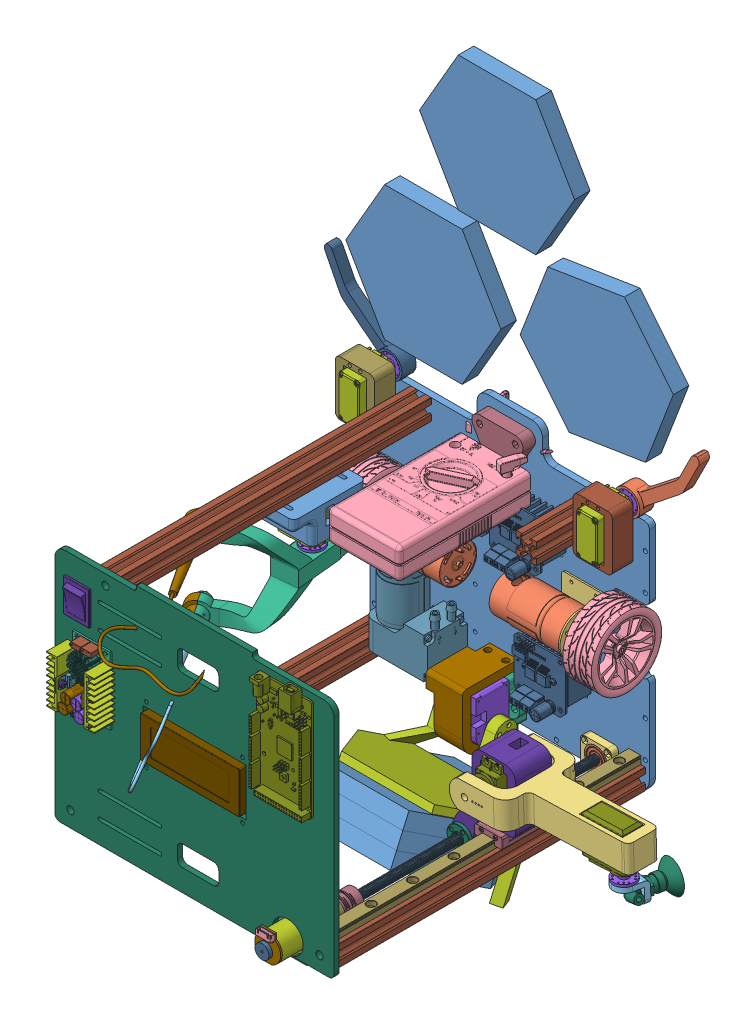
SolidWorks assembly conception_grand_robot_version_final, configuration Default. Lengths in mm. (continued)
Components (placement in the parent): (continued)
- XL4016E1 8A Buck Converter.STEP-1: XL4016E1 8A Buck Converter.STEP [Default] at (24.7028 162.9333 532.7888) x (0 1 0) z (1 0 0) size (65.3 28.6 46.4)
  - 8A Buck Converter PCB.STEP-1: 8A Buck Converter PCB.STEP [Default] at origin size (65.3 1.67 36.5)
  - Heat Exchanger.STEP-1: Heat Exchanger.STEP [Default] at (0 1.65 23.2) size (46 25.1 10.55)
  - Heat Exchanger.STEP-2: Heat Exchanger.STEP [Default] at (0 1.65 -23.2) x (-1 0 0) z (0 0 -1) size (46 25.1 10.55)
  - LargeGreen1000uF 35V Electrolytic Capacitor.STEP-1: LargeGreen1000uF 35V Electrolytic Capacitor.STEP [Default] at (-17.6782 1.65 7.8366) x (0 0 -1) z (1 0 0) size (9.9 26.01 9.9)
  - LargeGreen1000uF 35V Electrolytic Capacitor.STEP-2: LargeGreen1000uF 35V Electrolytic Capacitor.STEP [Default] at (-8.0317 1.65 5.0694) x (0 0 -1) z (1 0 0) size (9.9 26.01 9.9)
  - LargeGreen470uF 35V Electrolytic Capacitor.STEP-1: LargeGreen470uF 35V Electrolytic Capacitor.STEP [Default] at (-17.6617 1.65 -7.7514) x (0 0 1) z (-1 0 0) size (9.9 26.01 9.9)
  - LargeGreen470uF 35V Electrolytic Capacitor.STEP-2: LargeGreen470uF 35V Electrolytic Capacitor.STEP [Default] at (-7.9869 1.65 -5.0151) x (0 0 1) z (-1 0 0) size (9.9 26.01 9.9)
  - Screw Terminal x2.STEP-1: Screw Terminal x2.STEP [Default] at (-9.5 0 12.7839) x (-1 0 0) z (0 0 -1) size (7.95 12.9 10)
  - Screw Terminal x2.STEP-2: Screw Terminal x2.STEP [Default] at (-9.5 0 2.7839) x (-1 0 0) z (0 0 -1) size (7.95 12.9 10)
  - TrimmerW103.STEP-1: TrimmerW103.STEP [Default] at (32.65 6.9 -4.9563) x (0 0 1) z (-1 0 0) size (9.5 15.15 4.8)
  - TrimmerW103.STEP-2: TrimmerW103.STEP [Default] at (32.65 6.9 5.0581) x (0 0 1) z (-1 0 0) size (9.5 15.15 4.8)
  - whiteLEDShortLeed.STEP-1: whiteLEDShortLeed.STEP [Default] at (-13.9989 2.65 -0.1564) x (-1 0 0) z (0 0 -1) size (3.4 13.35 3.4)
  - Schottky Diode 20A 45V STPS2045CT.STEP-1: Schottky Diode 20A 45V STPS2045CT.STEP [Default] at (-0.0419 13.7002 12.65) x (-0.999962 0.008727 0) z (-0.008727 -0.999962 0) size (10.22 3.95 22.6)
  - XL4016E1 8A Voltage Regulator.STEP-1: XL4016E1 8A Voltage Regulator.STEP [Default] at (0 13.7 -12.65) x (1 0 0) z (0 -1 0) size (10.22 3.95 22.6)
  - Coil for Convertor.STEP-1: Coil for Convertor.STEP [Default] at (14.3115 2.9157 0.0112) size (27.99 14.39 26.86)
  - Small Plastic Washer.STEP-1: Small Plastic Washer.STEP [Default] at (0 18.5 -11.95) x (1 0 0) z (0 -1 0) size (6.1 1 6.1)
  - Small Plastic Washer.STEP-2: Small Plastic Washer.STEP [Default] at (0 18.5 10.95) x (1 0 0) z (0 -1 0) size (6.1 1 6.1)
  - pan head cross recess screw_iso_ISO 7045 - M3 x 8 - Z - 8S.STEP-1: pan head cross recess screw_iso_ISO 7045 - M3 x 8 - Z - 8S.STEP [Default] at (0 18.5 -8.55) x (0 0 -1) z (0.923728 0.383049 0) size (10.36 5.6 5.6)
  - pan head cross recess screw_iso_ISO 7045 - M3 x 8 - Z - 8S.STEP-2: pan head cross recess screw_iso_ISO 7045 - M3 x 8 - Z - 8S.STEP [Default] at (0 18.5 8.55) x (0 0 1) z (-1 0 0) size (10.36 5.6 5.6)
  - 1.7mmSmdCeramicCapacitorbrown.STEP-1: 1.7mmSmdCeramicCapacitorbrown.STEP [Default] at (2.849 0.0574 -8.3522) x (-1 0 0) z (0 0 1) size (2.02 0.49 1.04)
  - smdChip8pin.STEP-1: smdChip8pin.STEP [Default] at (19.9049 -0.725 7.6791) x (1 0 0) z (0 0 -1) size (7.3 1.22 4.5)
  - tinyVoltageRegulator.STEP-1: tinyVoltageRegulator.STEP [Default] at (13.3487 0 4.1964) x (-1 0 0) z (0 0 1) size (2.75 0.7 2.1)
  - tinyVoltageRegulator.STEP-2: tinyVoltageRegulator.STEP [Default] at (20.3011 0 11.2685) x (0.999962 0 0.008727) z (0.008727 0 -0.999962) size (2.75 0.7 2.1)
  - TinyVoltageRegulatorAMS1112.STEP-1: TinyVoltageRegulatorAMS1112.STEP [Default] at (15.0739 0.203 -4.8321) x (0 0 -1) z (-1 0 0) size (4.07 1.22 4.96)
  - tinySMDResistor222.STEP-1: tinySMDResistor222.STEP [Default] at (21.8501 0.1177 -6.1765) x (0 0 -1) z (-1 0 0) size (1.52 0.38 0.79)
  - tinySMDResistor.STEP-1: tinySMDResistor.STEP [Default] at (19.9225 0.1177 -6.1853) x (0 0 -1) z (-1 0 0) size (1.52 0.37 0.79)
  - 1.7mmSmdCeramicCapacitorbrown.STEP-2: 1.7mmSmdCeramicCapacitorbrown.STEP [Default] at (24.1073 0.0574 -6.3061) x (0 0 -1) z (-1 0 0) size (2.02 0.49 1.04)
  - 1.7mmSmdCeramicCapacitorbrown.STEP-3: 1.7mmSmdCeramicCapacitorbrown.STEP [Default] at (16.3262 0.0574 0.9562) x (0 0 -1) z (-1 0 0) size (2.02 0.49 1.04)
  - 1.7mmSmdCeramicCapacitorbrown.STEP-4: 1.7mmSmdCeramicCapacitorbrown.STEP [Default] at (18.1093 0.0574 0.9562) x (0 0 -1) z (-1 0 0) size (2.02 0.49 1.04)
  - tinySMDResistor.STEP-2: tinySMDResistor.STEP [Default] at (19.9874 0.1177 1.1419) x (0 0 -1) z (-1 0 0) size (1.52 0.37 0.79)
  - tinySMDResistor.STEP-3: tinySMDResistor.STEP [Default] at (21.6733 0.1177 1.1419) x (0 0 -1) z (-1 0 0) size (1.52 0.37 0.79)
  - tinySMDResistor.STEP-4: tinySMDResistor.STEP [Default] at (23.3916 0.1177 1.1419) x (0 0 -1) z (-1 0 0) size (1.52 0.37 0.79)
  - 1.7mmSmdCeramicCapacitorbrown.STEP-5: 1.7mmSmdCeramicCapacitorbrown.STEP [Default] at (25.4211 0.0574 4.0139) x (0 0 -1) z (-1 0 0) size (2.02 0.49 1.04)
  - 1.7mmSmdCeramicCapacitorbrown.STEP-6: 1.7mmSmdCeramicCapacitorbrown.STEP [Default] at (27.3088 0.0574 4.0139) x (0 0 -1) z (-1 0 0) size (2.02 0.49 1.04)
  - 1.7mmSmdCeramicCapacitorbrown.STEP-7: 1.7mmSmdCeramicCapacitorbrown.STEP [Default] at (23.1777 0.0574 11.1322) x (0 0 -1) z (-1 0 0) size (2.02 0.49 1.04)
  - 1.7mmSmdCeramicCapacitorbrown.STEP-8: 1.7mmSmdCeramicCapacitorbrown.STEP [Default] at (20.6839 0.0574 9.112) x (-0.999962 0 -0.008727) z (-0.008727 0 0.999962) size (2.02 0.49 1.04)
  - tinySMDResistor.STEP-5: tinySMDResistor.STEP [Default] at (17.7351 0.1177 11.3427) x (0 0 -1) z (-1 0 0) size (1.52 0.37 0.79)
  - tinySMDResistor.STEP-6: tinySMDResistor.STEP [Default] at (16.0827 0.1177 11.3427) x (0 0 -1) z (-1 0 0) size (1.52 0.37 0.79)
  - tinySMDResistor.STEP-7: tinySMDResistor.STEP [Default] at (16.906 0.1177 9.0199) x (-0.999962 0 -0.008727) z (-0.008727 0 0.999962) size (1.52 0.37 0.79)
  - tinySMDResistor.STEP-8: tinySMDResistor.STEP [Default] at (25.3907 0.1177 9.8144) x (-0.999962 0 -0.008727) z (-0.008727 0 0.999962) size (1.52 0.37 0.79)
  - R010 Resistor SMD.STEP-1: R010 Resistor SMD.STEP [Default] at (-19.919 0 5.2469) x (0 0 -1) z (-1 0 0) size (6.7 0.52 3.1)
  - solder.STEP-1: solder.STEP [Default] at (-27.65 0 -7.4411) x (-0.837169 0 -0.546944) z (-0.546944 0 0.837169) size (1.17 0.65 1.17)
  - solder.STEP-2: solder.STEP [Default] at (-27.65 0 -2.711) x (-0.837169 0 -0.546944) z (-0.546944 0 0.837169) size (1.17 0.65 1.17)
  - solder.STEP-3: solder.STEP [Default] at (-27.65 0 2.537) x (-0.837169 0 -0.546944) z (-0.546944 0 0.837169) size (1.17 0.65 1.17)
  - solder.STEP-4: solder.STEP [Default] at (-27.65 0 7.3016) x (-0.837169 0 -0.546944) z (-0.546944 0 0.837169) size (1.17 0.65 1.17)
  - solder1.8.STEP-1: solder1.8.STEP [Default] at (-20.8987 0 -15.5519) x (-0.837169 0 -0.546944) z (-0.546944 0 0.837169) size (1.8 0.65 1.8)
  - solder1.8.STEP-2: solder1.8.STEP [Default] at (20.8325 0 -15.5519) x (-0.837169 0 -0.546944) z (-0.546944 0 0.837169) size (1.8 0.65 1.8)
  - solder1.8.STEP-3: solder1.8.STEP [Default] at (20.8325 0 15.5391) x (-0.837169 0 -0.546944) z (-0.546944 0 0.837169) size (1.8 0.65 1.8)
  - solder1.8.STEP-4: solder1.8.STEP [Default] at (-20.8987 0 15.5391) x (-0.837169 0 -0.546944) z (-0.546944 0 0.837169) size (1.8 0.65 1.8)
  - solder.STEP-5: solder.STEP [Default] at (30.4698 0 7.6228) x (-0.837169 0 -0.546944) z (-0.546944 0 0.837169) size (1.17 0.65 1.17)
  - solder.STEP-6: solder.STEP [Default] at (30.4698 0 2.537) x (-0.837169 0 -0.546944) z (-0.546944 0 0.837169) size (1.17 0.65 1.17)
  - solder.STEP-7: solder.STEP [Default] at (30.4698 0 -2.454) x (-0.837169 0 -0.546944) z (-0.546944 0 0.837169) size (1.17 0.65 1.17)
  - solder.STEP-8: solder.STEP [Default] at (30.4698 0 -7.4732) x (-0.837169 0 -0.546944) z (-0.546944 0 0.837169) size (1.17 0.65 1.17)
  - solder.STEP-9: solder.STEP [Default] at (30.4698 0 -4.9355) x (-0.837169 0 -0.546944) z (-0.546944 0 0.837169) size (1.17 0.65 1.17)
  - solder.STEP-10: solder.STEP [Default] at (30.4698 0 5.0529) x (-0.837169 0 -0.546944) z (-0.546944 0 0.837169) size (1.17 0.65 1.17)
  - solder1.8.STEP-5: solder1.8.STEP [Default] at (1.0959 0 2.1506) x (-0.837169 0 -0.546944) z (-0.546944 0 0.837169) size (1.8 0.65 1.8)
  - solder1.8.STEP-6: solder1.8.STEP [Default] at (8.9457 0 2.3519) x (-0.837169 0 -0.546944) z (-0.546944 0 0.837169) size (1.8 0.65 1.8)
  - solder.STEP-11: solder.STEP [Default] at (-3.9931 0 -10.2017) x (-0.837169 0 -0.546944) z (-0.546944 0 0.837169) size (1.17 0.65 1.17)
  - solder.STEP-12: solder.STEP [Default] at (-1.9931 0 -10.2017) x (-0.837169 0 -0.546944) z (-0.546944 0 0.837169) size (1.17 0.65 1.17)
  - solder.STEP-13: solder.STEP [Default] at (0.0069 0 -10.2017) x (-0.837169 0 -0.546944) z (-0.546944 0 0.837169) size (1.17 0.65 1.17)
  - solder.STEP-14: solder.STEP [Default] at (2.0069 0 -10.2017) x (-0.837169 0 -0.546944) z (-0.546944 0 0.837169) size (1.17 0.65 1.17)
  - solder.STEP-15: solder.STEP [Default] at (4.0069 0 -10.2017) x (-0.837169 0 -0.546944) z (-0.546944 0 0.837169) size (1.17 0.65 1.17)
  - solder.STEP-16: solder.STEP [Default] at (-2.7433 0 10.0764) x (-0.873283 0 -0.487214) z (-0.487214 0 0.873283) size (1.17 0.65 1.17)
  - solder.STEP-17: solder.STEP [Default] at (-0.2033 0 10.0764) x (-0.873283 0 -0.487214) z (-0.487214 0 0.873283) size (1.17 0.65 1.17)
  - solder.STEP-18: solder.STEP [Default] at (2.3367 0 10.0764) x (-0.873283 0 -0.487214) z (-0.487214 0 0.873283) size (1.17 0.65 1.17)
  - solder.STEP-19: solder.STEP [Default] at (-8.0296 0 7.8897) x (-0.873283 0 -0.487214) z (-0.487214 0 0.873283) size (1.17 0.65 1.17)
  - solder.STEP-20: solder.STEP [Default] at (-8.0296 0 2.259) x (-0.873283 0 -0.487214) z (-0.487214 0 0.873283) size (1.17 0.65 1.17)
  - solder.STEP-21: solder.STEP [Default] at (-8.0296 0 -2.2341) x (-0.873283 0 -0.487214) z (-0.487214 0 0.873283) size (1.17 0.65 1.17)
  - solder.STEP-22: solder.STEP [Default] at (-8.0296 0 -7.8634) x (-0.873283 0 -0.487214) z (-0.487214 0 0.873283) size (1.17 0.65 1.17)
  - solder.STEP-23: solder.STEP [Default] at (-17.6872 0 -10.549) x (-0.873283 0 -0.487214) z (-0.487214 0 0.873283) size (1.17 0.65 1.17)
  - solder.STEP-24: solder.STEP [Default] at (-17.6872 0 -4.9388) x (-0.873283 0 -0.487214) z (-0.487214 0 0.873283) size (1.17 0.65 1.17)
  - solder.STEP-25: solder.STEP [Default] at (-17.6872 0 10.6333) x (-0.873283 0 -0.487214) z (-0.487214 0 0.873283) size (1.17 0.65 1.17)
  - solder.STEP-26: solder.STEP [Default] at (-17.6872 0 5.0231) x (-0.873283 0 -0.487214) z (-0.487214 0 0.873283) size (1.17 0.65 1.17)
  - solder.STEP-27: solder.STEP [Default] at (-15.2798 0 -0.193) x (-0.873283 0 -0.487214) z (-0.487214 0 0.873283) size (1.17 0.65 1.17)
  - solder.STEP-28: solder.STEP [Default] at (-12.7921 0 -0.193) x (-0.873283 0 -0.487214) z (-0.487214 0 0.873283) size (1.17 0.65 1.17)
- couvercle_support_sonde-1: couvercle_support_sonde [Default] at (-0.2607 219.7833 401.8495) x (0 1 0) z (0.846069 0 -0.533074) size (23.66 29.03 11.83)
- couvercle_support_sonde-2: couvercle_support_sonde [Default] at (-0.2607 149.7833 401.8495) x (0 1 0) z (0.846069 0 -0.533074) size (23.66 29.03 11.83)
- pince lamen_left1-1: pince lamen_left1 [Default] at (7.9528 266.0833 220.7888) x (-0.78692 0.617055 0) z (0 0 1) size (105.33 28.11 13.75)
Mates (geometry in assembly coordinates):
- Coincident1: coincident anti-aligned: plane of base-1 through (122.9528 157.5833 227.7888) normal (0 0 1); plane of assemblage_motor_complet-1/BAse motor-1 through (29.9528 137.5833 227.7888) normal (0 0 -1)
- Parallel1: parallel aligned: plane of base-1 through (-12.0472 287.5833 227.7888) normal (-1 0 0); plane of assemblage_motor_complet-1/BAse motor-1 through (28.4528 157.5833 253.7888) normal (-1 0 0)
- Width1: width anti-aligned: plane of Servo-1 through (103.2028 44.5833 260.7888) normal (-1 0 0); plane of Servo-1 through (142.7028 44.5833 260.7888) normal (1 0 0); plane of pince 3-1 through (103.7073 59.0854 266.418) normal (1 0 0); plane of pince 3-1 through (142.1984 59.0854 266.418) normal (-1 0 0)
- Concentric6: concentric aligned: cylinder of pince 3-1 through (122.9528 44.5833 260.7888) axis (1 0 0) radius 11; cylinder of Servo-1 through (103.2028 44.5833 260.7888) axis (1 0 0) radius 9.5
- Parallel5: parallel anti-aligned: plane of base-1 through (122.9528 157.5833 221.7888) normal (0 0 -1); plane of TABLE_2021.step-1/BaseTable.step-1/Ground.step-1 through (-709.5472 -667.4167 212.7888) normal (0 0 1)
- Width4: width anti-aligned: plane of base-1 through (-12.0472 292.5833 225.7888) normal (-1 0 0); plane of base-1 through (257.9528 292.5833 225.7888) normal (1 0 0); plane of TABLE_2021.step-1/Distributeurs.step-1/Distributeur 2 Top_1.step-1/TasseauCote_1.step-1; plane of TABLE_2021.step-1/Distributeurs.step-1/Distributeur 2 Top_1.step-1/TasseauCote_1.step-2
- Coincident8: coincident anti-aligned: plane of base-1 through (-12.0472 22.5833 225.7888) normal (0 -1 0); plane of TABLE_2021.step-1/Distributeurs.step-1/Distributeur 2 Top_1.step-1/TasseauAvant_1.step-1
- Tangent2: tangent anti-aligned: cylinder of assemblage_motor_complet-1/wheel-1 through (-8.8849 157.5833 246.7888) axis (1 0 0) radius 34; plane of TABLE_2021.step-1/BaseTable.step-1/Ground.step-1 through (982.9528 -674.9167 212.7888) normal (0 0 1)
- Concentric7: concentric aligned: cylinder of base-1 through (61.9528 172.5833 221.7888) axis (0 0 1) radius 2; cylinder of assemblage_motor_complet-1/BAse motor-1 through (61.9528 172.5833 187.7888) axis (0 0 1) radius 1.5
- Width5: width anti-aligned: plane of base-1 through (257.9528 287.5833 227.7888) normal (1 0 0); plane of Servo-1 through (-12.0472 287.5833 227.7888) normal (-1 0 0); plane of base-1 through (106.7028 54.0833 260.7888) normal (-1 0 0); plane of Servo-1 through (139.2028 54.0833 260.7888) normal (1 0 0)
- Distance1: distance = 5 mm aligned: plane of Servo-1 through (106.7028 32.5833 244.7888) normal (0 -1 0); plane of base-1 through (-12.0472 27.5833 227.7888) normal (0 -1 0)
- Coincident10: coincident anti-aligned: plane of bille porteuse-1/Robot2015_support bille porteuse_arriere-1 through (122.9528 39.4366 244.7888) normal (0 0 1); plane of Servo-1 through (106.7028 75.5833 244.7888) normal (0 0 -1)
- Coincident11: coincident anti-aligned: plane of base-1 through (122.9528 157.5833 227.7888) normal (0 0 1); plane of bille porteuse-1/Robot2015_support bille porteuse_arriere-1 through (122.9528 39.4366 227.7888) normal (0 0 -1)
- Coincident12: coincident anti-aligned: plane of Servo-1 through (106.7028 75.5833 276.7888) normal (0 0 1); plane of support_servo-1 through (134.2028 42.5727 276.7888) normal (0 0 -1)
- Coincident13: coincident aligned: plane of Servo-1 through (106.7028 54.0833 260.7888) normal (-1 0 0); plane of support_servo-1 through (106.7028 41.7493 266.8228) normal (-1 0 0)
- Concentric8: concentric anti-aligned: cylinder of base-1 through (122.9528 261.0833 221.7888) axis (0 0 1) radius 17; cylinder of bille porteuse-1/BillePorteuse-1 through (122.9528 52.5833 216.2888) axis (0 0 -1) radius 15.5
- Coincident17: coincident aligned: plane of bille porteuse-1/Robot2015_support bille porteuse_arriere-1 through (106.7028 32.5833 239.7888) normal (-1 0 0); plane of Servo-1 through (106.7028 54.0833 260.7888) normal (-1 0 0)
- Coincident23: coincident anti-aligned: plane of Servo-1 through (106.7028 75.5833 244.7888) normal (0 1 0); plane of support_servo-1 through (134.2028 75.5833 276.7888) normal (0 -1 0)
- Coincident24: coincident anti-aligned: plane of bille porteuse-1/Robot2015_support bille porteuse_arriere-1 through (139.2028 32.5833 239.7888) normal (0 -1 0); plane of support_servo-1 through (134.2028 32.5833 230.9626) normal (0 1 0)
- Concentric9: concentric aligned: cylinder of bille porteuse-1/Robot2015_support bille porteuse_arriere-1 through (122.9528 54.0833 239.7888) axis (0 0 -1) radius 11.9; cylinder of BillePorteuse-1 through (122.9528 54.0833 212.7888) axis (0 0 -1) radius 15.5
- Coincident26: coincident anti-aligned: plane of base-1 through (122.9528 157.5833 227.7888) normal (0 0 1); plane of system element de jeu vertical_vf-1/FORSETI_PERFIL_20x20_V-SLOT-1 through (250.0528 40.0795 227.7888) normal (0 0 -1)
- Distance2: distance = 4 mm aligned: plane of system element de jeu vertical-1/FORSETI_PERFIL_20x20_V-SLOT-1 through (234.3528 31.5833 227.7888) normal (0 -1 0); plane of base-1 through (-12.0472 27.5833 227.7888) normal (0 -1 0)
- Distance3: distance = 4 mm aligned: plane of system element de jeu vertical-1/FORSETI_PERFIL_20x20_V-SLOT-1 through (253.9528 51.1833 227.7888) normal (1 0 0); plane of base-1 through (257.9528 287.5833 227.7888) normal (1 0 0)
- Coincident29: coincident anti-aligned: plane of hexagone-1 through (122.9528 -3.9451 309.3699) normal (0 -0.91506 0.403318); plane of hexagone-2 through (122.9528 -3.9451 309.3699) normal (0 0.91506 -0.403318)
- Coincident30: coincident anti-aligned: plane of hexagone-2 through (122.9528 -17.671 315.4196) normal (0 -0.91506 0.403318); plane of hexagone-3 through (122.9528 -17.671 315.4196) normal (0 0.91506 -0.403318)
- Coincident31: coincident anti-aligned: plane of hexagone-1 through (122.9528 -3.9451 309.3699) normal (0 -0.91506 0.403318); plane of hexagone-2 through (122.9528 -3.9451 309.3699) normal (0 0.91506 -0.403318)
- Coincident32: coincident aligned: plane of hexagone-1 through (197.9528 -3.9451 309.3699) normal (0.866025 0.201659 0.45753); plane of hexagone-2 through (160.4528 22.2512 368.8047) normal (0.866025 0.201659 0.45753)
- Coincident33: coincident aligned: plane of hexagone-1 through (160.4528 -30.1414 249.935) normal (0.866025 -0.201659 -0.45753); plane of hexagone-2 through (197.9528 -3.9451 309.3699) normal (0.866025 -0.201659 -0.45753)
- Coincident34: coincident aligned: plane of hexagone-2 through (197.9528 -3.9451 309.3699) normal (0.866025 -0.201659 -0.45753); plane of hexagone-3 through (160.4528 -57.5932 262.0345) normal (0.866025 -0.201659 -0.45753)
- Coincident35: coincident aligned: plane of hexagone-2 through (85.4528 22.2512 368.8047) normal (0 0.403318 0.91506); plane of hexagone-3 through (160.4528 -5.2006 380.9043) normal (0 0.403318 0.91506)
- Width6: width anti-aligned: plane of hexagone-1 through (160.4528 -30.1414 249.935) normal (0.866025 -0.201659 -0.45753); plane of pince 3-1 through (47.9528 -3.9451 309.3699) normal (-0.866025 -0.201659 -0.45753); plane of hexagone-1 through (180.1984 -57.5255 299.3796) normal (-0.858356 0.206924 0.469475); plane of pince 3-1 through (65.7073 -57.5255 299.3796) normal (0.858356 0.206924 0.469475)
- Coincident36: coincident anti-aligned: plane of pince 3-1 through (122.9528 -18.4476 239.2747) normal (0 -0.91506 0.403318); plane of hexagone-1 through (122.9528 9.7808 303.3201) normal (0 0.91506 -0.403318)
- Coincident39: coincident: line of pince 3-1 through (180.1984 -57.5255 299.3796) axis (0 0.91506 -0.403318); plane of hexagone-3 through (160.4528 -57.5932 262.0345) normal (0.866025 -0.201659 -0.45753)
- Lock1: lock: unknown of pince 3-1; unknown of hexagone-1
- Coincident40: coincident anti-aligned: plane of base-1 through (122.9528 157.5833 227.7888) normal (0 0 1); plane of roulement-1 through (213.1252 52.5833 227.7888) normal (0 0 -1)
- Concentric11: concentric aligned: cylinder of system element de jeu vertical-1/12V 350RPM Small DFRobot Motor v8.step-1/Body_Back.step-1 through (213.1252 41.5833 550.5096) axis (0 0 -1) radius 12.5; cylinder of roulement-1 through (213.1252 41.5833 231.2888) axis (0 0 -1) radius 4
- Concentric12: concentric anti-aligned: cylinder of roulement-1 through (213.1252 41.5833 231.2888) axis (0 0 -1) radius 11; cylinder of support_roullement-1 through (213.1252 41.5833 227.7888) axis (0 0 1) radius 11.1
- Parallel8: parallel anti-aligned: plane of base-1 through (257.9528 287.5833 227.7888) normal (1 0 0); plane of support_roullement-1 through (198.1252 41.5833 227.7888) normal (-1 0 0)
- Coincident42: coincident anti-aligned: plane of base-1 through (122.9528 157.5833 227.7888) normal (0 0 1); plane of support_roullement-1 through (213.1252 41.5833 227.7888) normal (0 0 -1)
- Distance6: distance = 40 mm anti-aligned: plane of TABLE_2021.step-1/BaseTable.step-1/BorderLong.step-2 through (-17.0472 -674.9167 236.7888) normal (1 0 0); plane of base-1 through (-12.0472 287.5833 227.7888) normal (0 1 0)
- Concentric13: concentric aligned: circle of sonde --1; cylinder of support_sonde-1 through (-0.2607 149.7833 401.8495) axis (-0.533074 0 -0.846069) radius 7.8293
- Coincident53: coincident anti-aligned: plane of sonde --1 through (5.061 157.2738 409.59) normal (-0.533074 0 -0.846069); plane of support_sonde-1 through (4.7427 154.7833 409.7906) normal (0.533074 0 0.846069)
- Parallel15: parallel anti-aligned: plane of base-1 through (-12.0472 287.5833 227.7888) normal (-1 0 0); plane of TABLE_2021.step-1/BaseTable.step-1/BorderLong.step-2 through (-17.0472 -674.9167 236.7888) normal (1 0 0)
- Width7: width aligned: plane of TABLE_2021.step-1/CarreFouille.step-1/CarreFouilleTresorJaune.step-1/CarreFouille_1.step-1/SQUARE.step-1 through (-62.5404 82.5833 291.7012) normal (0 -1 0); plane of TABLE_2021.step-1/CarreFouille.step-1/CarreFouilleTresorJaune.step-1/CarreFouille_1.step-1/SQUARE.step-1 through (-62.5404 232.5833 291.7012) normal (0 1 0); plane of base-1 through (-12.0472 27.5833 227.7888) normal (0 -1 0); plane of base-1 through (-12.0472 287.5833 227.7888) normal (0 1 0)
- Distance7: distance = 5 mm anti-aligned: plane of TABLE_2021.step-1/BaseTable.step-1/BorderLong.step-2 through (-17.0472 -674.9167 236.7888) normal (1 0 0); plane of base-1 through (-12.0472 287.5833 227.7888) normal (-1 0 0)
- Concentric16: concentric anti-aligned: cylinder of support_sonde-1 through (46.9528 179.2833 342.7888) axis (0 -1 0) radius 10.5; cylinder of piece de liaison cercle MG996r-1 through (46.9528 192.2833 342.7888) axis (0 1 0) radius 10.375
- Coincident66: coincident anti-aligned: plane of support_sonde-1 through (33.0372 192.2833 329.092) normal (0 1 0); plane of piece de liaison cercle MG996r-1 through (46.9528 192.2833 342.7888) normal (0 -1 0)
- Coincident67: coincident anti-aligned: plane of support_sonde-1 through (4.7427 214.7833 409.7906) normal (0.533074 0 0.846069); plane of sonde +-2 through (-1.0468 216.713 413.4383) normal (-0.533074 0 -0.846069)
- Concentric17: concentric aligned: circle of support_sonde-1; circle of sonde +-2
- Coincident69: coincident anti-aligned: plane of base-1 through (122.9528 157.5833 227.7888) normal (0 0 1); plane of FORSETI_PERFIL_20x20_V-SLOT-4 through (202.8528 246.0795 227.7888) normal (0 0 -1)
- Distance10: distance = 30 mm aligned: plane of FORSETI_PERFIL_20x20_V-SLOT-4 through (199.3528 257.5833 527.7888) normal (0 1 0); plane of base-1 through (-12.0472 287.5833 227.7888) normal (0 1 0)
- Coincident99: coincident anti-aligned: plane of base-1 through (122.9528 157.5833 227.7888) normal (0 0 1); plane of FORSETI_PERFIL_20x20_V-SLOT-5 through (-3.1472 41.0795 227.7888) normal (0 0 -1)
- Distance23: distance = 5 mm aligned: plane of base-1 through (-12.0472 287.5833 227.7888) normal (-1 0 0); plane of FORSETI_PERFIL_20x20_V-SLOT-5 through (-7.0472 52.1833 527.7888) normal (-1 0 0)
- Distance24: distance = 5 mm aligned: plane of FORSETI_PERFIL_20x20_V-SLOT-5 through (-6.6472 32.5833 527.7888) normal (0 -1 0); plane of base-1 through (-12.0472 27.5833 227.7888) normal (0 -1 0)
- Parallel21: parallel aligned: plane of base-1 through (122.9528 157.5833 227.7888) normal (0 0 1); plane of IBT-2 (module only)-1 through (152.4528 207.7333 252.3888) normal (0 0 1)
- Coincident103: coincident anti-aligned: plane of base-1 through (122.9528 157.5833 227.7888) normal (0 0 1); plane of IBT-2 (module only)-1 through (177.9528 225.9083 227.7888) normal (0 0 -1)
- Distance25: distance = 80 mm aligned: plane of IBT-2 (module only)-1 through (177.9528 225.9083 250.7888) normal (1 0 0); plane of base-1 through (257.9528 287.5833 227.7888) normal (1 0 0)
- Distance26: distance = 55 mm aligned: plane of IBT-2 (module only)-1 through (174.7028 232.5833 252.3888) normal (0 1 0); plane of base-1 through (-12.0472 287.5833 227.7888) normal (0 1 0)
- Distance28: distance = 10 mm aligned: plane of Servo noir-3 through (247.9528 274.0833 236.5888) normal (1 0 0); plane of base-1 through (257.9528 287.5833 227.7888) normal (1 0 0)
- Coincident109: coincident anti-aligned: plane of Servo noir-3 through (237.9528 266.0833 231.0888) normal (0 0 -1); plane of piece de liaison cercle MG996r-3 through (237.9528 266.0833 231.0888) normal (0 0 1)
- Concentric24: concentric anti-aligned: cylinder of Servo noir-3 through (237.9528 266.0833 227.5888) axis (0 0 1) radius 3; cylinder of piece de liaison cercle MG996r-3 through (237.9528 266.0833 231.0888) axis (0 0 -1) radius 4.4
- Width10: width anti-aligned: plane of Servo noir-3 through (245.9528 236.0833 236.5888) normal (0 -1 0); plane of Servo noir-3 through (245.9528 276.0833 236.5888) normal (0 1 0); plane of support_servo_pince_lamen_imin-1 through (226.9528 235.0833 262.5888) normal (0 1 0); plane of support_servo_pince_lamen_imin-1 through (226.9528 277.0833 262.5888) normal (0 -1 0)
- Width11: width aligned: plane of Servo noir-3 through (247.9528 274.0833 236.5888) normal (1 0 0); plane of Servo noir-3 through (227.9528 274.0833 236.5888) normal (-1 0 0); plane of support_servo_pince_lamen_imin-1 through (226.9528 277.0833 262.5888) normal (1 0 0); plane of support_servo_pince_lamen_imin-1 through (248.9528 277.0833 262.5888) normal (-1 0 0)
- Coincident118: coincident anti-aligned: plane of FORSETI_PERFIL_20x20_V-SLOT-4 through (218.9528 257.1833 527.7888) normal (1 0 0); plane of support_servo_pince_lamen_imin-1 through (218.9528 282.5833 262.5888) normal (-1 0 0)
- Coincident119: coincident anti-aligned: plane of Servo noir-3 through (230.2644 280.7717 242.5888) normal (0 0 1); plane of support_servo_pince_lamen_imin-1 through (237.9528 256.0833 242.5888) normal (0 0 -1)
- Coincident121: coincident anti-aligned: plane of Servo noir-4 through (0.2644 280.7717 242.5888) normal (0 0 1); plane of support_servo_pince_lamen_isar-2 through (7.9528 256.0833 242.5888) normal (0 0 -1)
- Width17: width anti-aligned: plane of Servo noir-4 through (-2.0472 274.0833 236.5888) normal (-1 0 0); plane of Servo noir-4 through (17.9528 274.0833 236.5888) normal (1 0 0); plane of support_servo_pince_lamen_isar-2 through (-3.0472 235.0833 262.5888) normal (1 0 0); plane of support_servo_pince_lamen_isar-2 through (18.9528 235.0833 262.5888) normal (-1 0 0)
- Coincident127: coincident anti-aligned: plane of base-1 through (122.9528 157.5833 227.7888) normal (0 0 1); plane of support_scroll_arriere_robot_principale-1 through (122.9528 241.0833 227.7888) normal (0 0 -1)
- Concentric25: concentric anti-aligned: cylinder of base-1 through (122.9528 261.0833 221.7888) axis (0 0 1) radius 17; cylinder of support_scroll_arriere_robot_principale-1 through (122.9528 261.0833 239.7888) axis (0 0 -1) radius 11.9
- Parallel22: parallel aligned: plane of base-1 through (-12.0472 287.5833 227.7888) normal (0 1 0); plane of support_scroll_arriere_robot_principale-1 through (140.2733 278.5833 239.7888) normal (0 1 0)
- Concentric26: concentric aligned: cylinder of support_scroll_arriere_robot_principale-1 through (122.9528 261.0833 239.7888) axis (0 0 -1) radius 11.9; cylinder of BillePorteuse-2 through (122.9528 261.0833 214.7888) axis (0 0 -1) radius 12
- Tangent6: tangent aligned: sphere of BillePorteuse-1
- Distance33: distance = 2 mm: sphere of assembly; plane of assembly; sphere of BillePorteuse-2
- Coincident129: coincident aligned: plane of hexagone-4 through (39.3577 348.5402 212.7888) normal (0 0 -1)
- Coincident130: coincident aligned: plane of hexagone-4 through (39.3577 348.5402 212.7888) normal (0 0 -1); plane of hexagone-5 through (206.98 365.24 212.7888) normal (0 0 -1)
- Coincident132: coincident aligned: plane of hexagone-4 through (39.3577 348.5402 212.7888) normal (0 0 -1); plane of hexagone-6 through (110.587 492.7153 212.7888) normal (0 0 -1)
- Coincident141: coincident anti-aligned: plane of base-1 through (122.9528 157.5833 227.7888) normal (0 0 1); plane of PompeVide-AirpoD2028B-12vdc-1 through (19.441 93.4012 227.7888) normal (0 0 -1)
- Parallel23: parallel aligned: plane of base-1 through (-12.0472 27.5833 227.7888) normal (0 -1 0); plane of PompeVide-AirpoD2028B-12vdc-1 through (19.441 54.4012 266.3888) normal (0 -1 0)
- Concentric27: concentric anti-aligned: cylinder of base-1 through (196.4975 82.643 221.7888) axis (0 0 1) radius 1.75; cylinder of IBT-2 (module only)-3 through (196.4975 82.643 252.3888) axis (0 0 -1) radius 1.5
- Parallel24: parallel aligned: plane of base-1 through (257.9528 287.5833 227.7888) normal (1 0 0); plane of IBT-2 (module only)-3 through (201.2475 123.8531 252.3888) normal (1 0 0)
- Tangent7: tangent anti-aligned: plane of base-1 through (122.9528 157.5833 227.7888) normal (0 0 1); cylinder of IBT-2 (module only)-3 through (200.9975 119.668 228.7888) axis (0 -1 0) radius 1
- Coincident147: coincident anti-aligned: plane of FORSETI_PERFIL_20x20_V-SLOT-5 through (-3.1472 41.0795 527.7888) normal (0 0 1); plane of roof-1 through (122.9528 157.5833 527.7888) normal (0 0 -1)
- Coincident150: coincident aligned: plane of base-1 through (-12.0472 27.5833 227.7888) normal (0 -1 0); plane of roof-1 through (-12.0472 27.5833 532.7888) normal (0 -1 0)
- Coincident151: coincident aligned: plane of base-1 through (257.9528 287.5833 227.7888) normal (1 0 0); plane of roof-1 through (257.9528 287.5833 532.7888) normal (1 0 0)
- Coincident156: coincident anti-aligned: plane of roof-1 through (122.9528 157.5833 532.7888) normal (0 0 1); plane of Arduino Mega 2560-1 through (184.5366 251.2333 532.7888) normal (0 0 -1)
- Parallel25: parallel aligned: plane of roof-1 through (257.9528 287.5833 532.7888) normal (1 0 0); plane of Arduino Mega 2560-1 through (237.9528 149.6333 532.7888) normal (1 0 0)
- Coincident161: coincident anti-aligned: plane of roof-1 through (122.9528 157.5833 532.7888) normal (0 0 1); plane of interrupteur principal-1 through (10.4528 221.5833 532.7888) normal (0 0 -1)
- Distance35: distance = 10 mm aligned: plane of interrupteur principal-1 through (-2.0472 237.5833 534.7888) normal (-1 0 0); plane of roof-1 through (-12.0472 287.5833 532.7888) normal (-1 0 0)
- Distance36: distance = 20 mm aligned: plane of interrupteur principal-1 through (-2.0472 237.5833 534.7888) normal (0 1 0); plane of roof-1 through (122.9528 257.5833 532.7888) normal (0 1 0)
- Width21: width aligned: plane of 20x4 LCD.step-2 through (74.9528 162.5833 527.7888) normal (-1 0 0); plane of roof-1 through (170.9528 122.5833 527.7888) normal (1 0 0); plane of 20x4 LCD.step-2 through (-12.0472 287.5833 532.7888) normal (-1 0 0); plane of roof-1 through (257.9528 287.5833 532.7888) normal (1 0 0)
- Width22: width aligned: plane of 20x4 LCD.step-2 through (74.9528 122.5833 527.7888) normal (0 -1 0); plane of roof-1 through (170.9528 162.5833 527.7888) normal (0 1 0); plane of 20x4 LCD.step-2 through (-12.0472 27.5833 532.7888) normal (0 -1 0); plane of roof-1 through (122.9528 257.5833 532.7888) normal (0 1 0)
- Coincident168: coincident anti-aligned: plane of roof-1 through (122.9528 157.5833 527.7888) normal (0 0 -1); plane of 20x4 LCD.step-2 through (122.9528 142.5833 527.7888) normal (0 0 1)
- Coincident169: coincident aligned: plane of roof-1 through (122.9528 257.5833 532.7888) normal (0 1 0); plane of Arduino Mega 2560-1 through (228.6818 257.5833 545.2348) normal (0 1 0)
- Distance37: distance = 20 mm aligned: plane of Arduino Mega 2560-1 through (237.9528 149.6333 532.7888) normal (1 0 0); plane of roof-1 through (257.9528 287.5833 532.7888) normal (1 0 0)
- Concentric28: concentric anti-aligned: cylinder of Servo noir-1 through (46.9528 191.0833 342.7888) axis (0 1 0) radius 3; cylinder of piece de liaison cercle MG996r-1 through (46.9528 197.5833 342.7888) axis (0 -1 0) radius 4.4
- Coincident173: coincident anti-aligned: plane of Servo noir-1 through (46.9528 194.5833 342.7888) normal (0 -1 0); plane of piece de liaison cercle MG996r-1 through (46.9528 194.5833 342.7888) normal (0 1 0)
- Width25: width anti-aligned: plane of support_servo_sonde-1 through (57.9528 237.5833 331.7888) normal (0 0 1); plane of Servo noir-1 through (57.9528 237.5833 353.7888) normal (0 0 -1); plane of support_servo_sonde-1 through (54.9528 200.0833 332.7888) normal (0 0 -1); plane of Servo noir-1 through (54.9528 200.0833 352.7888) normal (0 0 1)
- Width26: width anti-aligned: plane of Servo noir-1 through (56.9528 200.0833 350.7888) normal (1 0 0); plane of support_servo_sonde-1 through (16.9528 200.0833 350.7888) normal (-1 0 0); plane of Servo noir-1 through (57.9528 237.5833 353.7888) normal (-1 0 0); plane of support_servo_sonde-1 through (15.9528 237.5833 353.7888) normal (1 0 0)
- Coincident179: coincident anti-aligned: plane of Servo noir-1 through (61.6412 206.0833 335.1004) normal (0 1 0); plane of support_servo_sonde-1 through (36.9528 206.0833 342.7888) normal (0 -1 0)
- Parallel30: parallel anti-aligned: plane of base-1 through (122.9528 157.5833 227.7888) normal (0 0 1); plane of Servo noir-1 through (54.9528 200.0833 332.7888) normal (0 0 -1)
- Coincident182: coincident anti-aligned: plane of FORSETI_PERFIL_20x20_V-SLOT-6 through (27.3528 237.5833 227.7888) normal (0 -1 0); plane of support_servo_sonde-1 through (36.9528 237.5833 342.7888) normal (0 1 0)
- Width27: width anti-aligned: plane of support_servo_sonde-1 through (9.9528 237.5833 359.7888) normal (-1 0 0); plane of support_servo_sonde-1 through (63.9528 237.5833 359.7888) normal (1 0 0); plane of FORSETI_PERFIL_20x20_V-SLOT-6 through (46.9528 237.9833 227.7888) normal (1 0 0); plane of FORSETI_PERFIL_20x20_V-SLOT-6 through (26.9528 257.1833 227.7888) normal (-1 0 0)
- Distance39: distance = 105 mm anti-aligned: plane of Servo noir-1 through (54.9528 200.0833 332.7888) normal (0 0 -1); plane of base-1 through (122.9528 157.5833 227.7888) normal (0 0 1)
- Coincident185: coincident anti-aligned: plane of piece de liaison cercle MG996r-3 through (237.9528 266.0833 225.7888) normal (0 0 -1); plane of pince lamen_write-4 through (237.9528 266.0833 225.7888) normal (0 0 1)
- Concentric30: concentric aligned: cylinder of piece de liaison cercle MG996r-3 through (237.9528 266.0833 225.7888) axis (0 0 1) radius 10.375; cylinder of pince lamen_write-4 through (237.9528 266.0833 215.7888) axis (0 0 1) radius 12.5
- Concentric31: concentric anti-aligned: cylinder of system element de jeu vertical_vf-1/kiso-1 through (243.9528 103.8333 380.6949) axis (0 0 -1) radius 2.92; cylinder of ServoAttacment2-1 through (243.9528 103.8333 376.6949) axis (0 0 1) radius 4
- Coincident186: coincident anti-aligned: plane of system element de jeu vertical_vf-1/kiso-1 through (243.9528 103.8333 380.6949) normal (0 0 1); plane of ServoAttacment2-1 through (243.9528 103.8333 380.6949) normal (0 0 -1)
- Coincident188: coincident aligned: plane of ServoAttacment2-1 through (243.9528 103.8333 380.6949) normal (0.029357 -0.999569 0)
- Coincident189: coincident anti-aligned: plane of Assemblage-1/piece servo2-2 through (232.3832 -1.7527 382.6949) normal (0 0 -1); plane of ServoAttacment2-1 through (243.9528 103.8333 382.6949) normal (0 0 1)
- Concentric32: concentric aligned: cylinder of Assemblage-1/piece servo2-2 through (243.9528 103.8333 392.6949) axis (0 0 -1) radius 14.6644; cylinder of ServoAttacment2-1 through (243.9528 103.8333 382.6949) axis (0 0 -1) radius 7
- Concentric33: concentric anti-aligned: cylinder of Assemblage-1/kiso-2 through (361.3502 77.9086 355.6949) axis (-0.029357 0.999569 0) radius 2.92; cylinder of piece de liaison cercle MG996r-6 through (361.2621 80.9073 355.6949) axis (0.029357 -0.999569 0) radius 4.4
- Distance40: distance = 3 mm anti-aligned: plane of Assemblage-1/kiso-2 through (361.3502 77.9086 355.6949) normal (0.029357 -0.999569 0); plane of piece de liaison cercle MG996r-6 through (361.2621 80.9073 355.6949) normal (-0.029357 0.999569 0)
- Coincident191: coincident anti-aligned: plane of support_servo_ventouse-1 through (361.4177 75.6096 355.6949) normal (-0.029357 0.999569 0); plane of piece de liaison cercle MG996r-6 through (361.4177 75.6096 355.6949) normal (0.029357 -0.999569 0)
- Concentric37: concentric anti-aligned: cylinder of system element de jeu vertical_vf-1/ventouse_final-1 through (369.5379 62.8425 317.2192) axis (0.199049 0.005846 -0.979972) radius 6.5; cylinder of support_servo_ventouse-1 through (364.6519 62.699 341.2743) axis (-0.199049 -0.005846 0.979972) radius 6.6
- Coincident192: coincident anti-aligned: plane of system element de jeu vertical_vf-1/ventouse_final-1 through (364.6519 62.699 341.2743) normal (-0.199049 -0.005846 0.979972); plane of support_servo_ventouse-1 through (374.4331 75.9919 343.3404) normal (0.199049 0.005846 -0.979972)
- Concentric38: concentric anti-aligned: cylinder of support_servo_ventouse-1 through (361.4177 75.6096 355.6949) axis (0.029357 -0.999569 0) radius 10.3; cylinder of piece de liaison cercle MG996r-6 through (361.4177 75.6096 355.6949) axis (-0.029357 0.999569 0) radius 10.375
- Concentric39: concentric anti-aligned: cylinder of support_servo_ventouse-1 through (361.4177 75.6096 355.6949) axis (0.029357 -0.999569 0) radius 10.3; cylinder of piece de liaison cercle MG996r-6 through (361.4177 75.6096 355.6949) axis (-0.029357 0.999569 0) radius 10.375
- Coincident193: coincident anti-aligned: plane of roof-1 through (122.9528 157.5833 532.7888) normal (0 0 1); plane of XL4016E1 8A Buck Converter.STEP-1/8A Buck Converter PCB.STEP-1 through (24.7028 162.9333 532.7888) normal (0 0 -1)
- Distance41: distance = 10 mm anti-aligned: plane of XL4016E1 8A Buck Converter.STEP-1/8A Buck Converter PCB.STEP-1 through (42.9528 195.5833 534.4388) normal (0 1 0); plane of interrupteur principal-1 through (-2.0472 205.5833 534.7888) normal (0 -1 0)
- Distance42: distance = 20 mm aligned: plane of interrupteur principal-1 through (22.9528 237.5833 534.7888) normal (1 0 0); plane of XL4016E1 8A Buck Converter.STEP-1/8A Buck Converter PCB.STEP-1 through (42.9528 130.2833 534.4388) normal (1 0 0)
- Coincident195: coincident anti-aligned: plane of support_sonde-1 through (-0.2607 219.7833 401.8495) normal (-0.846069 0 0.533074); plane of couvercle_support_sonde-1 through (-0.2607 219.7833 401.8495) normal (0.846069 0 -0.533074)
- Coincident196: coincident aligned: cone of support_sonde-1 through (-1.5651 219.7833 399.7791) axis (0.533074 0 0.846069); cone of couvercle_support_sonde-1 through (-1.5651 219.7833 399.7791) axis (0.533074 0 0.846069)
- Coincident197: coincident anti-aligned: plane of support_sonde-1 through (-0.2607 149.7833 401.8495) normal (-0.846069 0 0.533074); plane of couvercle_support_sonde-2 through (-0.2607 149.7833 401.8495) normal (0.846069 0 -0.533074)
- Coincident198: coincident aligned: cone of support_sonde-1 through (-1.5651 149.7833 399.7791) axis (0.533074 0 0.846069); cone of couvercle_support_sonde-2 through (-1.5651 149.7833 399.7791) axis (0.533074 0 0.846069)
- Coincident199: coincident aligned: plane of support_servo_pince_lamen_imin-1 through (237.9528 256.0833 262.5888) normal (0 0 1); plane of support_servo_pince_lamen_isar-2 through (7.9528 256.0833 262.5888) normal (0 0 1)
- Width28: width anti-aligned: plane of Servo noir-4 through (15.9528 276.0833 236.5888) normal (0 1 0); plane of Servo noir-4 through (15.9528 236.0833 236.5888) normal (0 -1 0); plane of support_servo_pince_lamen_isar-2 through (18.9528 277.0833 262.5888) normal (0 -1 0); plane of support_servo_pince_lamen_isar-2 through (18.9528 235.0833 262.5888) normal (0 1 0)
- Distance44: distance = 8 mm aligned: plane of support_servo_pince_lamen_imin-1 through (218.9528 229.5833 262.5888) normal (0 -1 0); plane of FORSETI_PERFIL_20x20_V-SLOT-4 through (218.5528 237.5833 527.7888) normal (0 -1 0)
- Concentric40: concentric anti-aligned: cylinder of piece de liaison cercle MG996r-4 through (7.9528 266.0833 225.7888) axis (0 0 1) radius 10.375; cylinder of pince lamen_left1-1 through (7.9528 266.0833 229.5388) axis (0 0 -1) radius 10.5
- Coincident200: coincident anti-aligned: plane of piece de liaison cercle MG996r-4 through (7.9528 266.0833 225.7888) normal (0 0 -1); plane of pince lamen_left1-1 through (7.9528 266.0833 225.7888) normal (0 0 1)
- Distance45: distance = 3 mm anti-aligned: plane of pince lamen_left1-1 through (7.9528 266.0833 215.7888) normal (0 0 -1); plane of TABLE_2021.step-1/BaseTable.step-1/Ground.step-1 through (982.9528 -674.9167 212.7888) normal (0 0 1)
